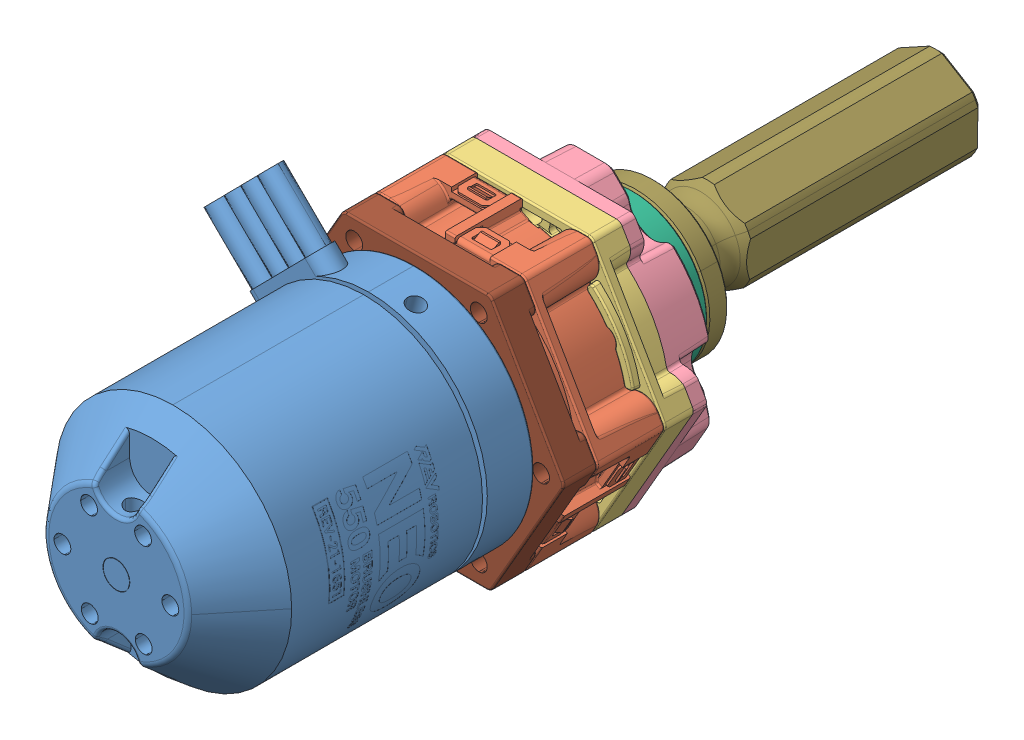
SolidWorks assembly ultraplanetary, configuration Default. Lengths in mm.
Overall size (63.81 63.81 121.86).
19 component instances, 12 part files, 14 mates.
Components (placement in the parent):
- REV-21-1651-1: REV-21-1651 [Default] at (0 19 -11.5) x (0 0 1) z (-0.999972 -0.007497 0) size (56.01 42.91 43.01)
- REV-41-1601-1: REV-41-1601 [Default] at (0 19 -10) x (-0.5 -0.866025 0) z (0 0 1) size (43.62 38.42 17.88)
- REV-41-1604-1: REV-41-1604 [Default] at (0 19 -26.25) x (-0.5 0.866025 0) z (0 0 1) size (54.69 56.73 18.25)
  - REV-41-1604.STEP-1: REV-41-1604.STEP [Default] at origin size (54.69 56.73 18.25)
    - REV-41-1604-2.STEP-1: REV-41-1604-2.STEP [Default] at origin size (43.57 38 6.25)
    - REV-41-1604-1.STEP-1: REV-41-1604-1.STEP [Default] at (0 0 7) x (0.5 0.866025 0) z (0 0 -1) size (43.57 38 7.03)
    - 6704ZZ.STEP-1: 6704ZZ.STEP [Default] at (0 0 7.75) x (0.995 -0.099871 0) z (0 0 1) size (27 27 4)
    - 6704ZZ.STEP-2: 6704ZZ.STEP [Default] at (0 0 3) x (0.993119 0.117109 0) z (0 0 1) size (27 27 4)
    - REV-40-1606_Through Hole.STEP-1: REV-40-1606_Through Hole.STEP [Default] at (0 0 10.95) x (-0.517794 -0.855505 0) z (0 0 -1) size (22 22 16.95)
    - REV-41-1604-4.STEP-1: REV-41-1604-4.STEP [Default] at (0 0 9.7) x (0.517794 0.855505 0) z (0 0 1) size (22 22 1.25)
    - REV-41-1604-3.STEP-1: REV-41-1604-3.STEP [Default] at (0 0 5) size (27.02 27 1.12)
    - socket head cap screw_am_B18.3.1M - 2 x 0.4 x 4 Hex SHCS -- 4NHX.STEP-1: socket head cap screw_am_B18.3.1M - 2 x 0.4 x 4 Hex SHCS -- 4NHX.STEP [Default] at (-11.8435 -10.7579 11.2) x (0 0 -1) z (-0.492915 -0.870077 0) size (6 3.8 3.8)
    - socket head cap screw_am_B18.3.1M - 2 x 0.4 x 4 Hex SHCS -- 4NHX.STEP-2: socket head cap screw_am_B18.3.1M - 2 x 0.4 x 4 Hex SHCS -- 4NHX.STEP [Default] at (-3.3948 15.6357 11.2) x (0 0 -1) z (-0.934724 -0.355374 0) size (6 3.8 3.8)
    - socket head cap screw_am_B18.3.1M - 2 x 0.4 x 4 Hex SHCS -- 4NHX.STEP-3: socket head cap screw_am_B18.3.1M - 2 x 0.4 x 4 Hex SHCS -- 4NHX.STEP [Default] at (15.2383 -4.8778 11.2) x (0 0 -1) z (0.970727 -0.240185 0) size (6 3.8 3.8)
    - 91294A003_BLACK ALLOY STEEL FLAT-HEAD SOCKET CAP SCREW_91294A003.STEP-1: 91294A003_BLACK ALLOY STEEL FLAT-HEAD SOCKET CAP SCREW_91294A003.STEP [Default] at (6.5084 3.5803 10.95) size (4 4 5)
    - 91294A003_BLACK ALLOY STEEL FLAT-HEAD SOCKET CAP SCREW_91294A003.STEP-2: 91294A003_BLACK ALLOY STEEL FLAT-HEAD SOCKET CAP SCREW_91294A003.STEP [Default] at (-0.1535 -7.4266 10.95) size (4 4 5)
    - 91294A003_BLACK ALLOY STEEL FLAT-HEAD SOCKET CAP SCREW_91294A003.STEP-3: 91294A003_BLACK ALLOY STEEL FLAT-HEAD SOCKET CAP SCREW_91294A003.STEP [Default] at (-6.3549 3.8463 10.95) size (4 4 5)
- REV-41-1607-1: REV-41-1607 [Default] at (0 19 0) x (-1 0 0) z (0 -1 0) size (43.57 5 38.01)
- REV-41-1620-1: REV-41-1620 [Default] at (0 19 -32.25) x (0.876175 0.481992 0) z (0 0 1) size (22 22 46.85)
Mates (geometry in assembly coordinates):
- Coincident1: coincident aligned: plane of REV-41-1607-1 through (0 19 0) normal (0 0 1)
- Coincident3: coincident anti-aligned: plane of REV-41-1607-1 through (10.9697 0 -5) normal (0 -1 0)
- Coincident6: coincident: line of REV-41-1607-1 through (0 12.5 -5) axis (0 0 1)
- Concentric1: concentric aligned: cylinder of REV-21-1651-1 through (0 19 44.5) axis (0 0 1) radius 6.5; cylinder of REV-41-1607-1 through (0 19 -5) axis (0 0 1) radius 6.5
- Concentric4: concentric anti-aligned: cylinder of REV-41-1601-1 through (9.2376 35 -5) axis (0 0 1) radius 1.6; cylinder of REV-41-1607-1 through (9.2376 35 -5) axis (0 0 -1) radius 1.25
- Coincident9: coincident anti-aligned: plane of REV-21-1651-1 through (-0.0487 25.4998 0) normal (0 0 -1); plane of REV-41-1607-1 through (0 19 0) normal (0 0 1)
- Concentric6: concentric anti-aligned: cylinder of REV-41-1601-1 through (-18.4752 19 -5) axis (0 0 1) radius 1.6; cylinder of REV-41-1607-1 through (-18.4752 19 -5) axis (0 0 -1) radius 1.25
- Coincident11: coincident anti-aligned: plane of REV-41-1601-1 through (0 19 -5) normal (0 0 1); plane of REV-41-1607-1 through (0 19 -5) normal (0 0 -1)
- Concentric8: concentric anti-aligned: cylinder of REV-41-1601-1 through (-9.2376 35 -5) axis (0 0 1) radius 1.6; cylinder of REV-41-1604-1/REV-41-1604.STEP-1/REV-41-1604-2.STEP-1 through (-9.2376 35 -26.25) axis (0 0 -1) radius 1.6
- Concentric9: concentric anti-aligned: cylinder of REV-41-1601-1 through (-18.4752 19 -5) axis (0 0 1) radius 1.6; cylinder of REV-41-1604-1/REV-41-1604.STEP-1/REV-41-1604-2.STEP-1 through (-18.4752 19 -26.25) axis (0 0 -1) radius 1.6
- Coincident12: coincident anti-aligned: plane of REV-41-1601-1 through (0 19 -15) normal (0 0 -1); plane of REV-41-1604-1/REV-41-1604.STEP-1/REV-41-1604-2.STEP-1 through (0 19 -15) normal (0 0 1)
- Coincident19: coincident anti-aligned: plane of REV-41-1604-1/REV-41-1604.STEP-1/REV-40-1606_Through Hole.STEP-1 through (0 19 -32.25) normal (0 0 -1); plane of REV-41-1620-1 through (0 19 -32.25) normal (0 0 1)
- Concentric10: concentric aligned: cylinder of REV-41-1604-1/REV-41-1604.STEP-1/REV-40-1606_Through Hole.STEP-1 through (-3.8559 26.0094 -32.25) axis (0 0 -1) radius 1.25; cylinder of REV-41-1620-1 through (-3.8559 26.0094 -35.25) axis (0 0 -1) radius 1.7
- Concentric11: concentric aligned: cylinder of REV-41-1604-1/REV-41-1604.STEP-1/REV-40-1606_Through Hole.STEP-1 through (7.9983 18.8346 -32.25) axis (0 0 -1) radius 1.25; cylinder of REV-41-1620-1 through (7.9983 18.8346 -35.25) axis (0 0 -1) radius 1.7
